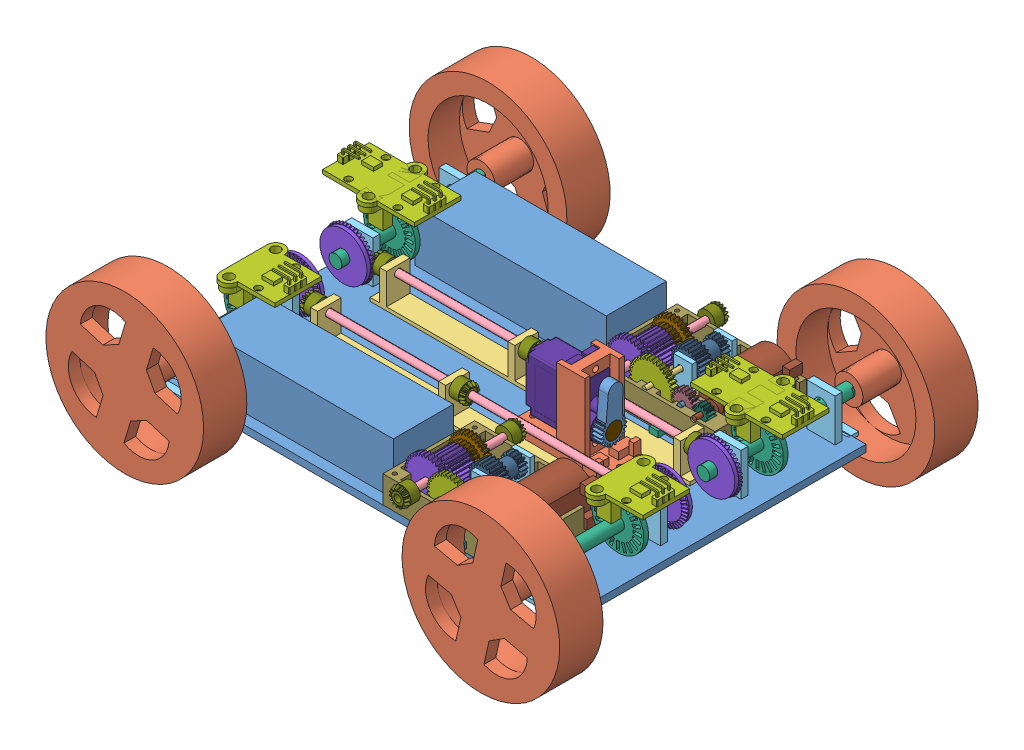
SolidWorks assembly 车子整体装配, configuration Default. Lengths in mm.
Overall size (247.94 92.49 177.76).
205 component instances, 52 part files, 49 mates.
Components (placement in the parent):
- 车底架-1: 车底架 [默认] at (0 0 0.6789) x (-1 0 0) z (0 1 0) size (180 125 25)
- 车轮-1: 车轮 [默认] at (-78.6398 14.5 66.1789) x (-0.472696 0.881226 0) z (0 0 1) size (67 67 21.38)
- 车轮-2: 车轮 [默认] at (-78.6398 14.5 -69.8211) x (0.905895 -0.423503 0) z (0 0 -1) size (67 67 21.38)
- 车轮-3: 车轮 [默认] at (77.7 14.5 -69.8211) x (-0.966558 0.256448 0) z (0 0 -1) size (67 67 21.38)
- 车轮-4: 车轮 [默认] at (77.7 14.5 71.1789) x (-0.843899 -0.536503 0) z (0 0 1) size (67 67 21.38)
- 垂直输出电机模组-2: 垂直输出电机模组 [默认] at (19.953 3 55.0825) x (-1 0 0) z (0 0 -1) size (59.95 25.43 55.83)
  - 连杆2-1: 连杆2 [默认] at (-14.147 11.5 28.863) x (1 0 0) z (0 1 0) size (2 36.3 2)
  - 连杆3-1: 连杆3 [默认] at (-1.947 11.5 34.6453) x (-1 0 0) z (0 -1 0) size (3 46 3)
  - 变速杆-1: 变速杆 [默认] at (-17.247 1.5 17.1537) x (1 0 0) z (0 1 0) size (14 21 14)
  - 变速杆固定横杆-1: 变速杆固定横杆 [默认] at (-23.247 4.1 14.4037) x (0 0 -1) z (0 -1 0) size (54 3.8 2.5)
  - 电机垂直传动齿轮2mm-1: 电机垂直传动齿轮2mm [默认] at (-14.147 11.5 5.0995) x (0 0 1) z (0.895442 0.445177 0) size (5.5 18.97 18.97)
    - 传动齿轮12x2-1: 传动齿轮12x2 [默认] at (-4.0458 0 0) x (0 0.164744 0.986336) z (-1 0 0) size (6.83 6.83 3) (hidden)
    - 36锥齿轮零件-1: 36锥齿轮零件 [默认] at origin size (5.5 18.97 18.97)
    - 圆柱齿轮36×2-1: 圆柱齿轮36×2 [默认] at (-7.0458 0 0) x (0 0.164744 0.986336) z (-1 0 0) size (18.96 18.96 2.5) (hidden)
  - 电机传动齿轮3mm-1: 电机传动齿轮3mm [默认] at (-0.2498 8.8187 -18.4418) x (0.429425 -0.903103 0) z (0 0 1) size (18.99 18.99 14.5)
    - 传动齿轮36x3-1: 传动齿轮36x3 [默认] at (-3.1503 -0.3813 16.7455) x (0.028836 -0.999584 0) z (0 0 1) size (18.96 18.96 5.5) (hidden)
    - 电机传动3mm-1: 电机传动3mm [默认] at origin size (18.99 18.99 14.5)
    - 圆柱齿轮24×3滑-1: 圆柱齿轮24×3滑 [默认] at (-3.1503 -0.3813 22.2455) x (0.028836 -0.999584 0) z (0 0 1) size (12.93 12.93 9) (hidden)
  - 电机固定传动齿轮3mm-1: 电机固定传动齿轮3mm [默认] at (-0.6653 10.9034 0.3109) x (-0.075925 -0.997114 0) z (0 0 1) size (17.17 17.17 5.51)
    - 传动齿轮24x3-1: 传动齿轮24x3 [默认] at (-0.4976 -1.3232 12.6928) x (0.102928 -0.994689 0) z (0 0 1) size (13.09 13.09 3.01) (hidden)
    - 圆柱齿轮32×3-1: 圆柱齿轮32×3 [默认] at (-0.4976 -1.3232 15.6928) x (-0.102928 0.994689 0) z (0 0 1) size (17.12 17.12 2.51) (hidden)
    - 齿轮24x32-1: 齿轮24x32 [默认] at origin size (17.17 17.17 5.51)
  - 电机滑动传动齿轮2mm-1: 电机滑动传动齿轮2mm [默认] at (-17.349 7.7022 27.4594) x (-0.972383 0.222908 -0.069163) z (0.122819 0.236734 -0.96378) size (13.39 14.37 17.14)
    - 传动齿轮24x2-1: 传动齿轮24x2 [默认] at (-1.0598 -0.2692 18.1158) x (-0.997571 -0.025895 0.064667) z (-0.069163 0.257573 -0.96378) size (13.09 13.09 11.75) (hidden)
    - 圆柱齿轮16×2-1: 圆柱齿轮16×2 [默认] at (-2.0799 3.53 3.9) x (-0.997571 -0.025895 0.064667) z (0.069163 -0.257573 0.96378) size (9.04 9.04 3.01) (hidden)
    - 齿轮32x24-1: 齿轮32x24 [默认] at origin size (13.39 14.37 17.14)
  - 电机-2: 电机 [默认] at (-35.547 11.5 26.9037) x (1 0 0) z (0 1 0) size (18 37.8 20)
  - 下壳2-1: 下壳2 [默认] at (-17.247 0 11.4037) size (59.5 13.5 39)
  - 圆柱齿轮18×2-1: 圆柱齿轮18×2 [默认] at (-27.847 11.5 -4.6963) size (10 9.9 3)
  - 连杆2短-1: 连杆2短 [默认] at (-27.847 11.5 -6.0963) x (0 -1 0) z (-1 0 0) size (2 6 2)
  - 上盖2-1: 上盖2 [默认] at (-17.247 23 11.4037) x (0 0 1) z (0 -1 0) size (39 57 16.5) (hidden)
  - 电机输出直齿轮12-1: 电机输出直齿轮12 [默认] at (-35.547 11.5 -4.6963) size (6.83 6.83 3)
  - 前后传动锥齿14-1: 前后传动锥齿14 [GB - Straight bevel pinion 0.5M14PT 42GT 20PA 2FW ---14O7.5H14MD3.0N] at (-1.947 11.5 35.1857) x (0 0 1) z (-0.999468 -0.032626 0) size (6.25 8.01 8.21)
  - 前后传动锥齿14-2: 前后传动锥齿14 [GB - Straight bevel pinion 0.5M14PT 42GT 20PA 2FW ---14O7.5H14MD3.0N] at (-1.947 11.5 -12.1697) x (0 0 -1) z (-0.993258 0.115929 0) size (6.25 8.01 8.21)
- 垂直输出电机模组-3: 垂直输出电机模组 [默认] at (19.953 3 -30.9175) x (-1 0 0) z (0 0 -1) size (59.95 25.43 55.83)
  - 连杆2-1: 连杆2 [默认] at (-14.147 11.5 28.863) x (1 0 0) z (0 1 0) size (2 36.3 2)
  - 连杆3-1: 连杆3 [默认] at (-1.947 11.5 34.6453) x (-1 0 0) z (0 -1 0) size (3 46 3)
  - 变速杆-1: 变速杆 [默认] at (-17.247 1.5 17.1537) x (1 0 0) z (0 1 0) size (14 21 14)
  - 变速杆固定横杆-1: 变速杆固定横杆 [默认] at (-23.247 4.1 14.4037) x (0 0 -1) z (0 -1 0) size (54 3.8 2.5)
  - 电机垂直传动齿轮2mm-1: 电机垂直传动齿轮2mm [默认] at (-14.147 11.5 5.0995) x (0 0 1) z (0.895442 0.445177 0) size (5.5 18.97 18.97)
    - 传动齿轮12x2-1: 传动齿轮12x2 [默认] at (-4.0458 0 0) x (0 0.164744 0.986336) z (-1 0 0) size (6.83 6.83 3) (hidden)
    - 36锥齿轮零件-1: 36锥齿轮零件 [默认] at origin size (5.5 18.97 18.97)
    - 圆柱齿轮36×2-1: 圆柱齿轮36×2 [默认] at (-7.0458 0 0) x (0 0.164744 0.986336) z (-1 0 0) size (18.96 18.96 2.5) (hidden)
  - 电机传动齿轮3mm-1: 电机传动齿轮3mm [默认] at (-0.2498 8.8187 -18.4418) x (0.429425 -0.903103 0) z (0 0 1) size (18.99 18.99 14.5)
    - 传动齿轮36x3-1: 传动齿轮36x3 [默认] at (-3.1503 -0.3813 16.7455) x (0.028836 -0.999584 0) z (0 0 1) size (18.96 18.96 5.5) (hidden)
    - 电机传动3mm-1: 电机传动3mm [默认] at origin size (18.99 18.99 14.5)
    - 圆柱齿轮24×3滑-1: 圆柱齿轮24×3滑 [默认] at (-3.1503 -0.3813 22.2455) x (0.028836 -0.999584 0) z (0 0 1) size (12.93 12.93 9) (hidden)
  - 电机固定传动齿轮3mm-1: 电机固定传动齿轮3mm [默认] at (-0.6653 10.9034 0.3109) x (-0.075925 -0.997114 0) z (0 0 1) size (17.17 17.17 5.51)
    - 传动齿轮24x3-1: 传动齿轮24x3 [默认] at (-0.4976 -1.3232 12.6928) x (0.102928 -0.994689 0) z (0 0 1) size (13.09 13.09 3.01) (hidden)
    - 圆柱齿轮32×3-1: 圆柱齿轮32×3 [默认] at (-0.4976 -1.3232 15.6928) x (-0.102928 0.994689 0) z (0 0 1) size (17.12 17.12 2.51) (hidden)
    - 齿轮24x32-1: 齿轮24x32 [默认] at origin size (17.17 17.17 5.51)
  - 电机滑动传动齿轮2mm-1: 电机滑动传动齿轮2mm [默认] at (-17.349 7.7022 27.4594) x (-0.972383 0.222908 -0.069163) z (0.122819 0.236734 -0.96378) size (13.39 14.37 17.14)
    - 传动齿轮24x2-1: 传动齿轮24x2 [默认] at (-1.0598 -0.2692 18.1158) x (-0.997571 -0.025895 0.064667) z (-0.069163 0.257573 -0.96378) size (13.09 13.09 11.75) (hidden)
    - 圆柱齿轮16×2-1: 圆柱齿轮16×2 [默认] at (-2.0799 3.53 3.9) x (-0.997571 -0.025895 0.064667) z (0.069163 -0.257573 0.96378) size (9.04 9.04 3.01) (hidden)
    - 齿轮32x24-1: 齿轮32x24 [默认] at origin size (13.39 14.37 17.14)
  - 电机-2: 电机 [默认] at (-35.547 11.5 26.9037) x (1 0 0) z (0 1 0) size (18 37.8 20)
  - 下壳2-1: 下壳2 [默认] at (-17.247 0 11.4037) size (59.5 13.5 39)
  - 圆柱齿轮18×2-1: 圆柱齿轮18×2 [默认] at (-27.847 11.5 -4.6963) size (10 9.9 3)
  - 连杆2短-1: 连杆2短 [默认] at (-27.847 11.5 -6.0963) x (0 -1 0) z (-1 0 0) size (2 6 2)
  - 上盖2-1: 上盖2 [默认] at (-17.247 23 11.4037) x (0 0 1) z (0 -1 0) size (39 57 16.5) (hidden)
  - 电机输出直齿轮12-1: 电机输出直齿轮12 [默认] at (-35.547 11.5 -4.6963) size (6.83 6.83 3)
  - 前后传动锥齿14-1: 前后传动锥齿14 [GB - Straight bevel pinion 0.5M14PT 42GT 20PA 2FW ---14O7.5H14MD3.0N] at (-1.947 11.5 35.1857) x (0 0 1) z (-0.999468 -0.032626 0) size (6.25 8.01 8.21)
  - 前后传动锥齿14-2: 前后传动锥齿14 [GB - Straight bevel pinion 0.5M14PT 42GT 20PA 2FW ---14O7.5H14MD3.0N] at (-1.947 11.5 -12.1697) x (0 0 -1) z (-0.993258 0.115929 0) size (6.25 8.01 8.21)
- 电池盒盖-1: 电池盒盖 [默认] at (29.863 2.9 -13.1084) x (0.999997 0 0.002262) z (0 -1 0) size (81 41 2.9) (hidden)
- SG舵机组合-1: SG舵机组合 [默认] at (30.9036 10.8514 6.7749) x (1 0 0) z (0 1 0) size (43 18.8 35.28)
  - SG90-1: SG90 [Default] at (-5.2804 6.096 11.2903) x (0 -1 0) z (0 0 1) size (12.19 30.42 32.28)
  - 舵机齿轮连接件-1: 舵机齿轮连接件 [默认] at (14.4676 6.096 6.096) x (0 0.047189 0.998886) z (-1 0 0) size (19.5 7 4)
  - 舵机齿轮连动件-1: 舵机齿轮连动件 [默认] at (10.4676 6.096 6.096) x (0 -0.047189 -0.998886) z (1 0 0) size (22.76 10.91 4)
  - 舵机底座-1: 舵机底座 [默认] at (0.7001 -2.0274 -7.8514) size (43 18.8 35.28)
- 四驱传动装配-1: 四驱传动装配 [默认] at (0 3 15.3675) x (-1 0 0) z (0 0 -1) size (140.66 16.17 10)
  - 四驱底座-1: 四驱底座 [默认] x (1 0 0) z (0 1 0) size (135.9 10 14.5)
  - 前后连接杆-1: 前后连接杆 [默认] at (70 11.5 0) x (0 0 1) z (0 -1 0) size (3 140 3)
  - 前后传动锥齿14-1: 前后传动锥齿14 [GB - Straight bevel pinion 0.5M14PT 42GT 20PA 2FW ---14O7.5H14MD3.0N] at (68.0747 11.5 0) size (6.25 8.01 8.21)
  - 前后传动锥齿14-2: 前后传动锥齿14 [GB - Straight bevel pinion 0.5M14PT 42GT 20PA 2FW ---14O7.5H14MD3.0N] at (-68.0747 11.5 0) x (-1 0 0) z (0 -0.988266 -0.152744) size (6.25 8.01 8.21)
  - 前后传动锥齿14-3: 前后传动锥齿14 [GB - Straight bevel pinion 0.5M14PT 42GT 20PA 2FW ---14O7.5H14MD3.0N] at (2.3282 11.5 0) x (-1 0 0) z (0 -0.992878 -0.119133) size (6.25 8.01 8.21)
- 四驱传动装配-2: 四驱传动装配 [默认] at (0 3 -14.0097) x (-1 0 0) z (0 0 -1) size (140.66 16.17 10)
  - 四驱底座-1: 四驱底座 [默认] x (1 0 0) z (0 1 0) size (135.9 10 14.5)
  - 前后连接杆-1: 前后连接杆 [默认] at (70 11.5 0) x (0 0 1) z (0 -1 0) size (3 140 3)
  - 前后传动锥齿14-1: 前后传动锥齿14 [GB - Straight bevel pinion 0.5M14PT 42GT 20PA 2FW ---14O7.5H14MD3.0N] at (68.0747 11.5 0) size (6.25 8.01 8.21)
  - 前后传动锥齿14-2: 前后传动锥齿14 [GB - Straight bevel pinion 0.5M14PT 42GT 20PA 2FW ---14O7.5H14MD3.0N] at (-68.0747 11.5 0) x (-1 0 0) z (0 -0.988266 -0.152744) size (6.25 8.01 8.21)
  - 前后传动锥齿14-3: 前后传动锥齿14 [GB - Straight bevel pinion 0.5M14PT 42GT 20PA 2FW ---14O7.5H14MD3.0N] at (2.3282 11.5 0) x (-1 0 0) z (0 -0.992878 -0.119133) size (6.25 8.01 8.21)
- 电路板.step-1: 电路板.step [默认] at (58.4777 38.0684 31.6949) x (-1 0 0) z (0 1 0) size (79.97 59.97 24.77) (hidden)
  - kw2D-U19.step-1: kw2D-U19.step [默认] at (12.0154 -45.4497 1.6001) x (-1 0 0) z (0 0 1) size (9.92 6.5 2.3)
    - TO-252-2_L6.5-W6.1-P4.58-LS10.0-TL.step-1: TO-252-2_L6.5-W6.1-P4.58-LS10.0-TL.step [默认] at origin size (9.92 6.5 2.3)
      - COMPOUND.step-1: COMPOUND.step [默认] at origin size (9.92 6.5 2.3)
  - kw2D-R20.step-1: kw2D-R20.step [默认] at (45.394 -23.6779 1.6001) x (0 1 0) z (0 0 1) size (2 1.3 0.61)
    - R0805.step-1: R0805.step [默认] at origin size (2 1.3 0.61)
      - COMPOUND-0.step-1: COMPOUND-0.step [默认] at origin size (2 1.3 0.61)
  - kw2D-R21.step-1: kw2D-R21.step [默认] at (36.3221 -51.4351 1.6001) size (2 1.3 0.61)
    - R0805.step-1: R0805.step [默认] at origin size (2 1.3 0.61)
      - COMPOUND-0.step-1: COMPOUND-0.step [默认] at origin size (2 1.3 0.61)
  - kw2D-R22.step-1: kw2D-R22.step [默认] at (36.4491 -46.7361 1.6001) x (0 -1 0) z (0 0 1) size (2 1.3 0.61)
    - R0805.step-1: R0805.step [默认] at origin size (2 1.3 0.61)
      - COMPOUND-0.step-1: COMPOUND-0.step [默认] at origin size (2 1.3 0.61)
  - kw2D-R19.step-1: kw2D-R19.step [默认] at (47.8791 -23.6779 1.6001) x (0 1 0) z (0 0 1) size (2 1.3 0.61)
    - R0805.step-1: R0805.step [默认] at origin size (2 1.3 0.61)
      - COMPOUND-0.step-1: COMPOUND-0.step [默认] at origin size (2 1.3 0.61)
  - kw2D-C1.step-1: kw2D-C1.step [默认] at (19.5072 -43.1801 1.6001) size (2 1.3 1.3)
    - C0805.step-1: C0805.step [默认] at origin size (2 1.3 1.3)
      - SOLID.step-1: SOLID.step [默认] at origin size (2 1.3 1.3)
  - kw2D-U18.step-1: kw2D-U18.step [默认] at (18.161 -27.9401 1.6001) x (0 1 0) z (0 0 1) size (20.2 9.89 24.27)
    - MULTIWATT-15_L19.6-W5.0-P1.27-L.step-1: MULTIWATT-15_L19.6-W5.0-P1.27-L.step [默认] at origin size (20.2 9.89 24.27)
      - COMPOUND-1.step-1: COMPOUND-1.step [默认] at origin size (20.2 9.89 24.27)
  - kw2D-SPD1.step-1: kw2D-SPD1.step [默认] at (80.3912 -43.1801 1.6001) x (0 1 0) z (0 0 1) size (10 5.7 10.5)
    - CONN-TH_3P-P2.54_2501S-3P.step-1: CONN-TH_3P-P2.54_2501S-3P.step [默认] at origin size (10 5.7 10.5)
      - COMPOUND-2.step-1: COMPOUND-2.step [默认] at origin size (10 5.7 10.5)
  - kw2D-DRI.step-1: kw2D-DRI.step [默认] at (80.3912 -6.731 1.6001) x (0 1 0) z (0 0 1) size (10 5.7 10.5)
    - CONN-TH_3P-P2.54_2501S-3P.step-1: CONN-TH_3P-P2.54_2501S-3P.step [默认] at origin size (10 5.7 10.5)
      - COMPOUND-2.step-1: COMPOUND-2.step [默认] at origin size (10 5.7 10.5)
  - kw2D-RST.step-1: kw2D-RST.step [默认] at (29.2863 -57.5565 1.6001) size (10 5.7 10.5)
    - CONN-TH_3P-P2.54_2501S-3P.step-1: CONN-TH_3P-P2.54_2501S-3P.step [默认] at origin size (10 5.7 10.5)
      - COMPOUND-2.step-1: COMPOUND-2.step [默认] at origin size (10 5.7 10.5)
  - kw2D-SPD2.step-1: kw2D-SPD2.step [默认] at (80.3912 -32.0041 1.6001) x (0 1 0) z (0 0 1) size (10 5.7 10.5)
    - CONN-TH_3P-P2.54_2501S-3P.step-1: CONN-TH_3P-P2.54_2501S-3P.step [默认] at origin size (10 5.7 10.5)
      - COMPOUND-2.step-1: COMPOUND-2.step [默认] at origin size (10 5.7 10.5)
  - kw2D-BAT1.step-1: kw2D-BAT1.step [默认] at (6.985 -53.8481 1.6001) x (0 1 0) z (0 0 1) size (7.5 5.9 10.6)
    - CONN-TH_2P-P2.50_HX25003-2A.step-1: CONN-TH_2P-P2.50_HX25003-2A.step [默认] at origin size (7.5 5.9 10.6)
      - COMPOUND-3.step-1: COMPOUND-3.step [默认] at origin size (7.5 5.9 10.6)
  - kw2D-MOT1.step-1: kw2D-MOT1.step [默认] at (18.034 -56.3881 1.6001) size (7.5 5.9 10.6)
    - CONN-TH_2P-P2.50_HX25003-2A.step-1: CONN-TH_2P-P2.50_HX25003-2A.step [默认] at origin size (7.5 5.9 10.6)
      - COMPOUND-3.step-1: COMPOUND-3.step [默认] at origin size (7.5 5.9 10.6)
  - kw2D-BAT2.step-1: kw2D-BAT2.step [默认] at (6.985 -6.223 1.6001) x (0 1 0) z (0 0 1) size (7.5 5.9 10.6)
    - CONN-TH_2P-P2.50_HX25003-2A.step-1: CONN-TH_2P-P2.50_HX25003-2A.step [默认] at origin size (7.5 5.9 10.6)
      - COMPOUND-3.step-1: COMPOUND-3.step [默认] at origin size (7.5 5.9 10.6)
  - kw2D-LIT.step-1: kw2D-LIT.step [默认] at (45.5169 -56.2865 1.6001) size (7.5 5.9 10.6)
    - CONN-TH_2P-P2.50_HX25003-2A.step-1: CONN-TH_2P-P2.50_HX25003-2A.step [默认] at origin size (7.5 5.9 10.6)
      - COMPOUND-3.step-1: COMPOUND-3.step [默认] at origin size (7.5 5.9 10.6)
  - kw2D-MOT2.step-1: kw2D-MOT2.step [默认] at (18.034 -5.207 1.6001) x (-1 0 0) z (0 0 1) size (7.5 5.9 10.6)
    - CONN-TH_2P-P2.50_HX25003-2A.step-1: CONN-TH_2P-P2.50_HX25003-2A.step [默认] at origin size (7.5 5.9 10.6)
      - COMPOUND-3.step-1: COMPOUND-3.step [默认] at origin size (7.5 5.9 10.6)
  - kw2D-U17.step-1: kw2D-U17.step [默认] at (43.6881 -46.4821 1.6001) x (-1 0 0) z (0 0 1) size (10.3 10 2.35)
    - SOP-16_L10.3-W7.5-P1.27-LS10.4-BL.step-1: SOP-16_L10.3-W7.5-P1.27-LS10.4-BL.step [默认] at origin size (10.3 10 2.35)
      - COMPOUND-4.step-1: COMPOUND-4.step [默认] at origin size (10.3 10 2.35)
  - kw2D-U20.step-1: kw2D-U20.step [默认] at (19.431 -47.7521 1.6001) size (1.62 0.81 0.45)
    - R0603.step-1: R0603.step [默认] at origin size (1.62 0.81 0.45)
      - COMPOUND-5.step-1: COMPOUND-5.step [默认] at origin size (1.62 0.81 0.45)
  - kw2D-U26.step-1: kw2D-U26.step [默认] at (24.13 -11.5398 1.6001) x (0 -1 0) z (0 0 1) size (5.1 2.7 2.2)
    - SMA_L4.5-W2.7-LS5.1-RD.step-1: SMA_L4.5-W2.7-LS5.1-RD.step [默认] at origin size (5.1 2.7 2.2)
      - COMPOUND-6.step-1: COMPOUND-6.step [默认] at origin size (5.1 2.7 2.2)
  - kw2D-U27.step-1: kw2D-U27.step [默认] at (20.193 -11.5398 1.6001) x (0 -1 0) z (0 0 1) size (5.1 2.7 2.2)
    - SMA_L4.5-W2.7-LS5.1-RD.step-1: SMA_L4.5-W2.7-LS5.1-RD.step [默认] at origin size (5.1 2.7 2.2)
      - COMPOUND-6.step-1: COMPOUND-6.step [默认] at origin size (5.1 2.7 2.2)
  - kw2D-U28.step-1: kw2D-U28.step [默认] at (27.8131 -11.5398 1.6001) x (0 -1 0) z (0 0 1) size (5.1 2.7 2.2)
    - SMA_L4.5-W2.7-LS5.1-RD.step-1: SMA_L4.5-W2.7-LS5.1-RD.step [默认] at origin size (5.1 2.7 2.2)
      - COMPOUND-6.step-1: COMPOUND-6.step [默认] at origin size (5.1 2.7 2.2)
  - kw2D-U30.step-1: kw2D-U30.step [默认] at (29.8027 -35.8141 1.6001) x (0 1 0) z (0 0 1) size (5.1 2.7 2.2)
    - SMA_L4.5-W2.7-LS5.1-RD.step-1: SMA_L4.5-W2.7-LS5.1-RD.step [默认] at origin size (5.1 2.7 2.2)
      - COMPOUND-6.step-1: COMPOUND-6.step [默认] at origin size (5.1 2.7 2.2)
  - kw2D-U29.step-1: kw2D-U29.step [默认] at (33.6551 -35.8141 1.6001) x (0 1 0) z (0 0 1) size (5.1 2.7 2.2)
    - SMA_L4.5-W2.7-LS5.1-RD.step-1: SMA_L4.5-W2.7-LS5.1-RD.step [默认] at origin size (5.1 2.7 2.2)
      - COMPOUND-6.step-1: COMPOUND-6.step [默认] at origin size (5.1 2.7 2.2)
  - kw2D-U32.step-1: kw2D-U32.step [默认] at (25.9504 -35.8141 1.6001) x (0 1 0) z (0 0 1) size (5.1 2.7 2.2)
    - SMA_L4.5-W2.7-LS5.1-RD.step-1: SMA_L4.5-W2.7-LS5.1-RD.step [默认] at origin size (5.1 2.7 2.2)
      - COMPOUND-6.step-1: COMPOUND-6.step [默认] at origin size (5.1 2.7 2.2)
  - kw2D-U31.step-1: kw2D-U31.step [默认] at (37.2111 -35.9411 1.6001) x (0 1 0) z (0 0 1) size (5.1 2.7 2.2)
    - SMA_L4.5-W2.7-LS5.1-RD.step-1: SMA_L4.5-W2.7-LS5.1-RD.step [默认] at origin size (5.1 2.7 2.2)
      - COMPOUND-6.step-1: COMPOUND-6.step [默认] at origin size (5.1 2.7 2.2)
  - kw2D-U25.step-1: kw2D-U25.step [默认] at (16.383 -11.5398 1.6001) x (0 -1 0) z (0 0 1) size (5.1 2.7 2.2)
    - SMA_L4.5-W2.7-LS5.1-RD.step-1: SMA_L4.5-W2.7-LS5.1-RD.step [默认] at origin size (5.1 2.7 2.2)
      - COMPOUND-6.step-1: COMPOUND-6.step [默认] at origin size (5.1 2.7 2.2)
  - kw2D-D1.step-1: kw2D-D1.step [默认] at (46.8631 -12.192 1.6001) x (0 -1 0) z (0 0 1) size (4.7 2.6 2.1)
    - SMA_L4.3-W2.6-LS5.2-RD.step-1: SMA_L4.3-W2.6-LS5.2-RD.step [默认] at origin size (4.7 2.6 2.1)
      - COMPOUND-7.step-1: COMPOUND-7.step [默认] at origin size (4.7 2.6 2.1)
  - kw2D-DIS1.step-1: kw2D-DIS1.step [默认] at (79.5022 -19.05 1.6001) x (0 -1 0) z (0 0 1) size (12.5 5.7 10)
    - CONN-TH_4P-P2.50_4PIN.step-1: CONN-TH_4P-P2.50_4PIN.step [默认] at origin size (12.5 5.7 10)
      - COMPOUND-8.step-1: COMPOUND-8.step [默认] at origin size (12.5 5.7 10)
  - kw2D-DIS2.step-1: kw2D-DIS2.step [默认] at (38.1001 -3.937 1.6001) x (-1 0 0) z (0 0 1) size (12.5 5.7 10)
    - CONN-TH_4P-P2.50_4PIN.step-1: CONN-TH_4P-P2.50_4PIN.step [默认] at origin size (12.5 5.7 10)
      - COMPOUND-8.step-1: COMPOUND-8.step [默认] at origin size (12.5 5.7 10)
  - kw2D-U38.step-1: kw2D-U38.step [默认] at (39.5479 -55.3213 1.6001) x (0 1 0) z (0 0 1) size (2.4 2.9 1.05)
    - SOT-23-3_L2.9-W1.3-P1.90-LS2.4.step-1: SOT-23-3_L2.9-W1.3-P1.90-LS2.4.step [默认] at origin size (2.4 2.9 1.05)
      - COMPOUND-9.step-1: COMPOUND-9.step [默认] at origin size (2.4 2.9 1.05)
  - kw2D-U21.step-1: kw2D-U21.step [默认] at (45.5931 -31.7501 1.6001) x (-1 0 0) z (0 0 1) size (6.23 4.5 7.6)
    - SW-TH_4P-L4.5-W4.5-P3.00-LS5.0.step-1: SW-TH_4P-L4.5-W4.5-P3.00-LS5.0.step [默认] at origin size (6.23 4.5 7.6)
      - COMPOUND-10.step-1: COMPOUND-10.step [默认] at origin size (6.23 4.5 7.6)
  - kw2D-U33.step-1: kw2D-U33.step [默认] at (37.9731 -19.05 1.6001) size (9.1 8.3 10.2)
    - CAP-SMD_BD8.0-L8.3-W8.3-LS9.1-FD.step-1: CAP-SMD_BD8.0-L8.3-W8.3-LS9.1-FD.step [默认] at origin size (9.1 8.3 10.2)
      - SOLID-11.step-1: SOLID-11.step [默认] at origin size (9.1 8.3 10.2)
  - Board.step-1: Board.step [默认] at origin size (79.97 59.97 1.6)
- 传动车轴组合-1: 传动车轴组合 [默认] at (-94.9182 72.5 46.6851) x (-1 0 0) z (0 -1 0) size (31.71 68 34.77)
  - 传动底座-1: 传动底座 [默认] at (-16.2784 8.3855 71) x (0 -1 0) z (0 0 -1) size (56 12 19.5)
  - 连杆3带齿轮-1: 连杆3带齿轮 [默认] at (-16.2784 -20.6366 58) size (22 68 22)
  - HC_020K-1: HC_020K [Varsayılan] at (-24.2034 16.3634 41.1) x (0 -1 0) z (0 0 1) size (27.15 23.16 17.67)
  - 42锥齿轮X5-1: 42锥齿轮X5 [GB - Straight bevel gear 0.5M 42GT 14PT 20PA 2FW ---42O20H6MD5.0N] at (-16.2784 35.4363 58) x (0 -1 0) z (-0.164767 0 0.986333) size (3.43 21.19 21.21)
- 传动车轴组合右-1: 传动车轴组合右 [默认] at (-78.6398 14.5 -62.2362) x (1 0 0) z (0 -1 0) size (31.71 68 34.77)
  - 传动车轴组合-1: 传动车轴组合 [默认] at (16.2784 16.9089 -58) size (31.71 68 34.77)
    - 传动底座-1: 传动底座 [默认] at (-16.2784 8.3855 71) x (0 -1 0) z (0 0 -1) size (56 12 19.5)
    - 连杆3带齿轮-1: 连杆3带齿轮 [默认] at (-16.2784 -20.6366 58) size (22 68 22)
    - HC_020K-1: HC_020K [Varsayılan] at (-24.2034 16.3634 41.1) x (0 -1 0) z (0 0 1) size (27.15 23.16 17.67)
    - 42锥齿轮X5-1: 42锥齿轮X5 [GB - Straight bevel gear 0.5M 42GT 14PT 20PA 2FW ---42O20H6MD5.0N] at (-16.2784 35.4363 58) x (0 -1 0) z (-0.164767 0 0.986333) size (3.43 21.19 21.21)
  - HC_020K-2: HC_020K [Varsayılan] at (7.925 33.2722 -16.9) x (0 1 0) z (0 0 1) size (27.15 23.16 17.67)
- 传动车轴组合-4: 传动车轴组合 [默认] at (61.4216 72.5 46.6851) x (-1 0 0) z (0 -1 0) size (31.71 68 34.77)
  - 传动底座-1: 传动底座 [默认] at (-16.2784 8.3855 71) x (0 -1 0) z (0 0 -1) size (56 12 19.5)
  - 连杆3带齿轮-1: 连杆3带齿轮 [默认] at (-16.2784 -20.6366 58) size (22 68 22)
  - HC_020K-1: HC_020K [Varsayılan] at (-24.2034 16.3634 41.1) x (0 -1 0) z (0 0 1) size (27.15 23.16 17.67)
  - 42锥齿轮X5-1: 42锥齿轮X5 [GB - Straight bevel gear 0.5M 42GT 14PT 20PA 2FW ---42O20H6MD5.0N] at (-16.2784 35.4363 58) x (0 -1 0) z (-0.164767 0 0.986333) size (3.43 21.19 21.21)
- 传动车轴组合右-2: 传动车轴组合右 [默认] at (77.7 14.5 -62.2362) x (1 0 0) z (0 -1 0) size (31.71 68 34.77)
  - 传动车轴组合-1: 传动车轴组合 [默认] at (16.2784 16.9089 -58) size (31.71 68 34.77)
    - 传动底座-1: 传动底座 [默认] at (-16.2784 8.3855 71) x (0 -1 0) z (0 0 -1) size (56 12 19.5)
    - 连杆3带齿轮-1: 连杆3带齿轮 [默认] at (-16.2784 -20.6366 58) size (22 68 22)
    - HC_020K-1: HC_020K [Varsayılan] at (-24.2034 16.3634 41.1) x (0 -1 0) z (0 0 1) size (27.15 23.16 17.67)
    - 42锥齿轮X5-1: 42锥齿轮X5 [GB - Straight bevel gear 0.5M 42GT 14PT 20PA 2FW ---42O20H6MD5.0N] at (-16.2784 35.4363 58) x (0 -1 0) z (-0.164767 0 0.986333) size (3.43 21.19 21.21)
  - HC_020K-2: HC_020K [Varsayılan] at (7.925 33.2722 -16.9) x (0 1 0) z (0 0 1) size (27.15 23.16 17.67)
- 18650-1: 18650 [默认] at (-61.0952 13.375 -44.5711) x (0 -0.540817 0.84114) z (0 0.84114 0.540817) size (18.25 67.5 18.25)
- 18650-2: 18650 [默认] at (-61.6368 13.375 45.9289) x (0 -0.315594 -0.948894) z (0 -0.948894 0.315594) size (18.25 67.5 18.25)
Mates (geometry in assembly coordinates):
- 重合2: coincident: plane of 车底架-1 through (0 0 0.6789) normal (0 -1 0)
- 距离3: distance = 3 mm anti-aligned: plane of 车轮-1 through (-78.6398 14.5 66.1789) normal (0 0 -1); plane of 车底架-1 through (90 3 63.1789) normal (0 0 1)
- 同心2: concentric anti-aligned: cylinder of 车轮-1 through (-78.6398 14.5 156.6838) axis (0 0 -1) radius 6; cylinder of 车轮-2 through (-78.6398 14.5 -160.326) axis (0 0 1) radius 6
- 距离6: distance = 5 mm anti-aligned: plane of 车轮-2 through (-78.6398 14.5 -66.8211) normal (0 0 1); plane of 车底架-1 through (90 3 -61.8211) normal (0 0 -1)
- 同心3: concentric anti-aligned: cylinder of 车轮-3 through (77.7 14.5 -160.326) axis (0 0 1) radius 6; cylinder of 车轮-4 through (77.7 14.5 161.6838) axis (0 0 -1) radius 6
- 距离7: distance = 5 mm anti-aligned: plane of 车轮-4 through (77.7 14.5 68.1789) normal (0 0 -1); plane of 车底架-1 through (90 3 63.1789) normal (0 0 1)
- 距离8: distance = 5 mm anti-aligned: plane of 车轮-3 through (77.7 14.5 -66.8211) normal (0 0 1); plane of 车底架-1 through (90 3 -61.8211) normal (0 0 -1)
- 重合4: coincident anti-aligned: plane of 车底架-1 through (0 3 0.6789) normal (0 1 0); plane of 垂直输出电机模组-2/下壳-1 through (50 3 32.0124) normal (0 -1 0)
- 距离18: distance = 12.3 mm: cylinder of 车轮-3 through (77.7 14.5 -160.326) axis (0 0 1) radius 6; plane of 车底架-1 through (90 3 63.1789) normal (1 0 0)
- 重合105: coincident: plane of 车底架-1 through (0 0 0.6789) normal (-1 0 0)
- 重合107: coincident aligned: plane of 车底架-1 through (0 0 0.6789) normal (0 -1 0); plane of 电池盒盖-1 through (29.863 0 -13.1084) normal (0 -1 0)
- 重合128: coincident anti-aligned: plane of 车底架-1 through (0 3 0.6789) normal (0 1 0); plane of 四驱传动装配-1/四驱底座-1 through (0 3 15.3675) normal (0 -1 0)
- 重合133: coincident aligned: plane of 垂直输出电机模组-2/连杆3-2 through (-70.1 14.5 16.3789) normal (0 -1 0); plane of 四驱传动装配-1/前后连接杆-1 through (-70 14.5 15.3675) normal (0 -1 0)
- 同心65: concentric aligned: cylinder of 垂直输出电机模组-2/连杆3-2 through (-8.9 14.5 16.3789) axis (-1 0 0) radius 1.5; cylinder of 四驱传动装配-1/前后连接杆-1 through (70 14.5 15.3675) axis (-1 0 0) radius 1.5
- 重合134: coincident aligned: plane of 四驱传动装配-1/前后连接杆-1 through (70 14.5 15.3675) normal (1 0 0); plane of 四驱传动装配-2/前后连接杆-1 through (70 14.5 -14.0097) normal (1 0 0)
- 重合140: coincident anti-aligned: plane of 车底架-1 through (0 3 0.6789) normal (0 1 0); plane of SG舵机组合-1/舵机底座-1 through (31.6037 3 8.8022) normal (0 -1 0)
- 平行2: parallel anti-aligned: plane of 车底架-1 through (0 3 0.6789) normal (0 1 0); plane of 电路板.step-1/Board.step-1 through (14.7946 38.0684 0.6789) normal (0 -1 0)
- 宽度2: width aligned: plane of 车底架-1 through (90 3 -61.8211) normal (0 0 -1); plane of 电路板.step-1/Board.step-1 through (90 3 63.1789) normal (0 0 1); plane of 车底架-1 through (-25.1928 38.0684 -29.3085) normal (0 0 -1); plane of 电路板.step-1/Board.step-1 through (54.782 38.0684 30.6662) normal (0 0 1)
- 距离19: distance = 0.1 mm anti-aligned: plane of 车底架-1 through (9.6 25 58.6789) normal (1 0 0); plane of 垂直输出电机模组-2/下壳2-1 through (9.7 14.5 63.1789) normal (-1 0 0)
- 宽度3: width aligned: plane of 车底架-1 through (90 3 -61.8211) normal (0 0 -1); plane of 车底架-1 through (90 3 63.1789) normal (0 0 1); plane of SG舵机组合-1/舵机底座-1 through (7.8711 5 -7.7211) normal (0 0 -1); plane of SG舵机组合-1/舵机底座-1 through (45.3711 5 9.0789) normal (0 0 1)
- 重合147: coincident aligned: plane of 车底架-1 through (90 3 63.1789) normal (0 0 1); plane of 垂直输出电机模组-2/下壳2-1 through (64.7 14.5 63.1789) normal (0 0 1)
- 重合148: coincident anti-aligned: plane of 车底架-1 through (0 3 0.6789) normal (0 1 0); plane of 四驱传动装配-2/四驱底座-1 through (0 3 -14.0097) normal (0 -1 0)
- 重合149: coincident anti-aligned: plane of 车底架-1 through (0 3 0.6789) normal (0 1 0); plane of 垂直输出电机模组-3/下壳2-1 through (37.2 3 -42.3211) normal (0 -1 0)
- 重合150: coincident aligned: plane of 垂直输出电机模组-2/下壳2-1 through (64.7 14.5 63.1789) normal (1 0 0); plane of 垂直输出电机模组-3/下壳2-1 through (64.7 14.5 -22.8211) normal (1 0 0)
- 重合151: coincident aligned: plane of 车底架-1 through (90 3 -61.8211) normal (0 0 -1); plane of 垂直输出电机模组-3/下壳2-1 through (64.7 14.5 -61.8211) normal (0 0 -1)
- 距离20: distance = 11.5 mm anti-aligned: plane of 传动车轴组合-1/连杆3带齿轮-1 through (-78.6398 14.5 67.3217) normal (0 -1 0); plane of 车底架-1 through (0 3 0.6789) normal (0 1 0)
- 宽度4: width aligned: plane of 车底架-1 through (-90 3 63.1789) normal (-1 0 0); plane of 四驱传动装配-1/四驱底座-1 through (90 3 63.1789) normal (1 0 0); plane of 车底架-1 through (-63.95 17.5 20.3675) normal (-1 0 0); plane of 四驱传动装配-1/四驱底座-1 through (63.95 17.5 20.3675) normal (1 0 0)
- 重合157: coincident aligned: plane of 传动车轴组合-1/连杆3带齿轮-1 through (-78.6398 14.5 67.3217) normal (0 -1 0); plane of 传动车轴组合右-1/连杆3带齿轮-1 through (-78.2202 14.5 -62.9506) normal (0 -1 0)
- 重合158: coincident anti-aligned: plane of 传动车轴组合-1/连杆3带齿轮-1 through (-78.6398 14.5 67.3217) normal (-1 0 0); plane of 传动车轴组合右-1/连杆3带齿轮-1 through (-78.2202 14.5 -62.9506) normal (1 0 0)
- 同心66: concentric anti-aligned: cylinder of 车轮-2 through (-78.6398 14.5 -160.326) axis (0 0 1) radius 6; cylinder of 传动车轴组合右-1/连杆3带齿轮-1 through (-78.2202 14.5 -1.9506) axis (0 0 -1) radius 2.75
- 宽度5: width anti-aligned: plane of 车底架-1 through (90 3 -61.8211) normal (0 0 -1); plane of 传动车轴组合右-1/连杆3带齿轮-1 through (90 3 63.1789) normal (0 0 1); plane of 车底架-1 through (-78.2202 14.5 -1.9506) normal (0 0 1); plane of 传动车轴组合-1/连杆3带齿轮-1 through (-78.6398 14.5 6.3217) normal (0 0 -1)
- 重合159: coincident aligned: plane of 传动车轴组合右-1/连杆3带齿轮-1 through (-78.2202 14.5 -1.9506) normal (0 0 1); plane of 传动车轴组合右-2/连杆3带齿轮-1 through (77.7 14.5 -1.9506) normal (0 0 1)
- 重合160: coincident aligned: plane of 传动车轴组合-1/连杆3带齿轮-1 through (-78.6398 14.5 6.3217) normal (0 0 -1); plane of 传动车轴组合-4/连杆3带齿轮-1 through (77.7 14.5 6.3217) normal (0 0 -1)
- 距离22: distance = 11.5 mm anti-aligned: plane of 传动车轴组合-4/连杆3带齿轮-1 through (77.7 14.5 67.3217) normal (0 -1 0); plane of 车底架-1 through (0 3 0.6789) normal (0 1 0)
- 重合161: coincident aligned: plane of 传动车轴组合-4/连杆3带齿轮-1 through (77.7 14.5 67.3217) normal (0 -1 0); plane of 传动车轴组合右-2/连杆3带齿轮-1 through (77.7 14.5 -62.9506) normal (0 -1 0)
- 重合162: coincident anti-aligned: plane of 传动车轴组合-4/连杆3带齿轮-1 through (77.7 14.5 67.3217) normal (-1 0 0); plane of 传动车轴组合右-2/连杆3带齿轮-1 through (77.7 14.5 -62.9506) normal (1 0 0)
- 同心67: concentric anti-aligned: cylinder of 车轮-4 through (77.7 14.5 161.6838) axis (0 0 -1) radius 6; cylinder of 传动车轴组合-4/连杆3带齿轮-1 through (77.7 14.5 6.3217) axis (0 0 1) radius 2.75
- 相切1: tangent anti-aligned: plane of 车底架-1 through (0 22.5 0.6789) normal (0 -1 0); cylinder of 18650-1 through (4.6048 13.375 -44.5711) axis (-1 0 0) radius 9.125
- 宽度6: width: plane of 车底架-1 through (-69.1 25.001 -54.8211) normal (0 0 1); plane of 18650-1 through (-69.1 25.001 -34.3211) normal (0 0 -1); cylinder of 车底架-1 through (4.6048 13.375 -44.5711) axis (-1 0 0) radius 9.125
- 相切2: tangent anti-aligned: plane of 车底架-1 through (0 22.5 0.6789) normal (0 -1 0); cylinder of 18650-2 through (4.0632 13.375 45.9289) axis (-1 0 0) radius 9.125
- 宽度7: width: plane of 车底架-1 through (-69.1 3.001 35.6789) normal (0 0 1); plane of 18650-2 through (-69.1 3.001 56.1789) normal (0 0 -1); cylinder of 车底架-1 through (4.0632 13.375 45.9289) axis (-1 0 0) radius 9.125
- 同心68: concentric anti-aligned: cylinder of 传动车轴组合-1/连杆3带齿轮-1 through (-78.6398 14.5 6.3217) axis (0 0 1) radius 2.75; cylinder of 传动车轴组合右-1/传动车轴组合-1/连杆3带齿轮-1 through (-78.6398 14.5 -4.964) axis (0 0 -1) radius 2.75
- 平行3: parallel anti-aligned: plane of 车底架-1 through (0 3 0.6789) normal (0 1 0); plane of 传动车轴组合右-1/传动车轴组合-1/连杆3带齿轮-1 through (-78.6398 14.5 -65.964) normal (0 -1 0)
- 同心69: concentric anti-aligned: cylinder of 车轮-2 through (-78.6398 14.5 -160.326) axis (0 0 1) radius 6; cylinder of 传动车轴组合右-1/传动车轴组合-1/连杆3带齿轮-1 through (-78.6398 14.5 -4.964) axis (0 0 -1) radius 2.75
- 宽度8: width anti-aligned: plane of 车底架-1 through (90 3 -61.8211) normal (0 0 -1); plane of 车底架-1 through (90 3 63.1789) normal (0 0 1); plane of 传动车轴组合右-1/传动车轴组合-1/连杆3带齿轮-1 through (-78.6398 14.5 -4.964) normal (0 0 1); plane of 传动车轴组合-1/连杆3带齿轮-1 through (-78.6398 14.5 6.3217) normal (0 0 -1)
- 同心70: concentric anti-aligned: cylinder of 传动车轴组合-4/连杆3带齿轮-1 through (77.7 14.5 6.3217) axis (0 0 1) radius 2.75; cylinder of 传动车轴组合右-2/传动车轴组合-1/连杆3带齿轮-1 through (77.7 14.5 -4.964) axis (0 0 -1) radius 2.75
- 平行4: parallel anti-aligned: plane of 车底架-1 through (0 3 0.6789) normal (0 1 0); plane of 传动车轴组合右-2/传动车轴组合-1/连杆3带齿轮-1 through (77.7 14.5 -65.964) normal (0 -1 0)
- 宽度9: width aligned: plane of 车底架-1 through (90 3 -61.8211) normal (0 0 -1); plane of 车底架-1 through (90 3 63.1789) normal (0 0 1); plane of 传动车轴组合-4/连杆3带齿轮-1 through (77.7 14.5 6.3217) normal (0 0 -1); plane of 传动车轴组合右-2/传动车轴组合-1/连杆3带齿轮-1 through (77.7 14.5 -4.964) normal (0 0 1)
- 宽度10: width aligned: plane of 车底架-1 through (90 3 63.1789) normal (0 0 1); plane of 四驱传动装配-1/四驱底座-1 through (90 3 -61.8211) normal (0 0 -1); plane of 车底架-1 through (67.95 4.5 20.3675) normal (0 0 1); plane of 四驱传动装配-2/四驱底座-1 through (67.95 4.5 -19.0097) normal (0 0 -1)
